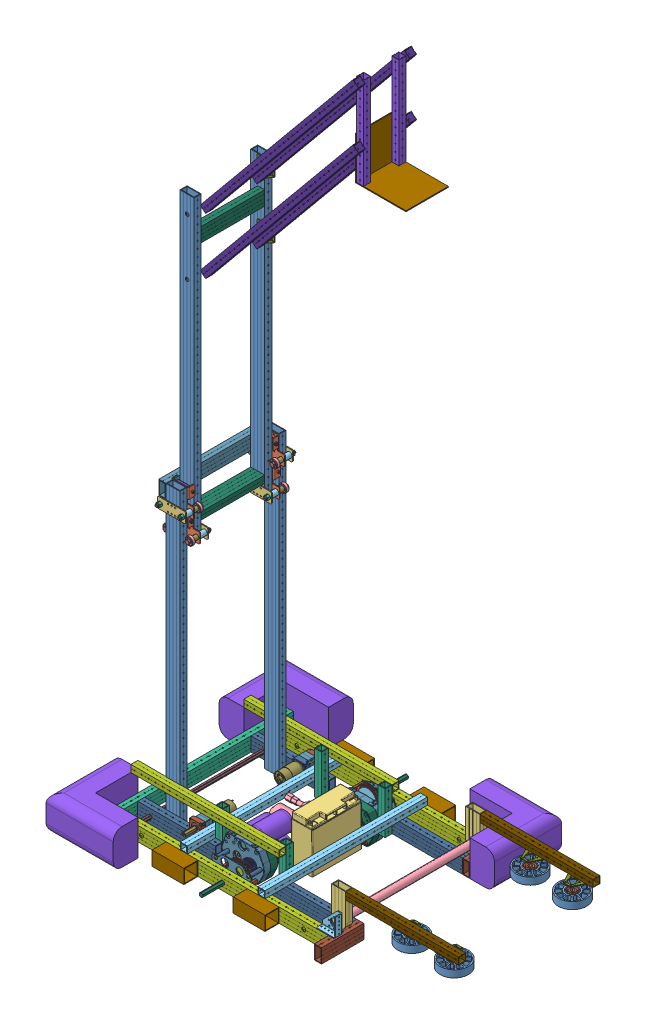
SolidWorks assembly Test Robot 2, configuration Default. Lengths in mm.
Overall size (1308.22 2664.65 863.6).
474 component instances, 122 part files, 52 mates.
Components (placement in the parent):
- Elevator Base Frame-1: Elevator Base Frame [Default] at (1458.6962 1126.0433 -272.9132) x (0 0 1) z (-1 0 0) size (419.1 1066.8 119.57)
  - Elevator Fixed Frame-1: Elevator Fixed Frame [Default] at (786.6435 8.8982 734.5957) x (1 0 0) z (0 1 0) size (25.4 50.8 1066.8)
  - Elevator Fixed Frame-2: Elevator Fixed Frame [Default] at (431.0435 8.8982 734.5957) x (1 0 0) z (0 1 0) size (25.4 50.8 1066.8)
  - am-3844+2x1+Elevator+Assembly+Example-1: am-3844+2x1+Elevator+Assembly+Example [Default] at (37.3435 1067.0077 761.7737) x (-1 0 0) z (0 0 1) size (82.37 89.82 113.91)
    - Example Single Corner Bearing Assembly-1: Example Single Corner Bearing Assembly [Default] at (-442.3285 289.2703 9.4128) x (0 0 1) z (-1 0 0) size (113.91 89.82 82.37)
      - Large Bearing Block Plate-1: Large Bearing Block Plate [Default] at (-85.6128 70.3392 -35.9285) x (1 0 0) z (0 -1 0) size (101.6 24.99 88.9)
      - Small Bearing Block Plate-1: Small Bearing Block Plate [Default] at (-85.6128 70.3392 -64.5035) x (1 0 0) z (0 -1 0) size (101.6 3.17 38.1)
      - 1614Z Bearing-1: 1614Z Bearing [Default] at (-74.6273 89.3892 -8.941) x (-0.590982 0.806685 0) z (0 0 1) size (28.58 28.58 9.53)
      - 1614Z Bearing-2: 1614Z Bearing [Default] at (5.0017 89.3892 -8.941) x (0.001674 0.999999 0) z (0 0 1) size (28.58 28.58 9.53)
      - AS75-18-64 Aluminum Spacer-1: AS75-18-64 Aluminum Spacer [Default] at (5.0017 89.3892 -35.9285) x (-0.668699 0.743533 0) z (-0.743533 -0.668699 0) size (19.05 25.41 19.05)
      - AS75-18-64 Aluminum Spacer-2: AS75-18-64 Aluminum Spacer [Default] at (-74.6273 89.3892 -61.3285) x (0.536222 0.844077 0) z (0.844077 -0.536222 0) size (19.05 25.41 19.05)
      - 3-8-16 NyLock Nut - Mcm 95615A140_95615A140-1: 3-8-16 NyLock Nut - Mcm 95615A140_95615A140 [Default] at (5.0017 89.3892 -64.5035) x (1 0 0) z (0 1 0) size (14.29 12 16.5)
      - 3-8-16 NyLock Nut - Mcm 95615A140_95615A140-2: 3-8-16 NyLock Nut - Mcm 95615A140_95615A140 [Default] at (-74.6273 89.3892 -64.5035) x (1 0 0) z (0 1 0) size (14.29 12 16.5)
      - am-0602 .250 x .192 x 2.14 Brass Tube-1: am-0602 .250 x .192 x 2.14 Brass Tube [Default] at (-7.6348 38.5892 -20.4599) x (0 0 1) z (-1 0 0) size (6.35 6.35 54.36)
      - 13RS075051 .750 x .260 x 1.00 Spacer-1: 13RS075051 .750 x .260 x 1.00 Spacer [Default] at (-60.2128 38.5892 -20.4599) x (0 -0.722855 0.691) z (0 0.691 0.722855) size (19.05 25.4 19.05)
      - 13RS075051 .750 x .260 x 1.00 Spacer-2: 13RS075051 .750 x .260 x 1.00 Spacer [Default] at (-34.8128 38.5892 -20.4599) x (0 -0.801304 -0.598258) z (0 -0.598258 0.801304) size (19.05 25.4 19.05)
      - 0.25 Flat Washer_Preferred Wide FW 0.25-1: 0.25 Flat Washer_Preferred Wide FW 0.25 [Default] at (-60.2128 38.5892 -20.4599) x (1 0 0) z (0 -0.116572 0.993182) size (1.4 15.88 15.88)
      - 0.25 Flat Washer_Preferred Wide FW 0.25-2: 0.25 Flat Washer_Preferred Wide FW 0.25 [Default] at (-8.0158 38.5892 -20.4599) size (1.4 15.88 15.88)
      - 10-32 Nylock Nut-1: 10-32 Nylock Nut [Default] at (-65.1658 38.5892 -20.4599) x (0 -0.097883 0.995198) z (-1 0 0) size (9.53 11 5.96)
      - SHCS 10-32 x 2.75_HX-SHCS 0.19-32x2.75x0.875-C-1: SHCS 10-32 x 2.75_HX-SHCS 0.19-32x2.75x0.875-C [Default] at (0.3662 38.5892 -20.4599) x (-1 0 0) z (0 0.982583 -0.185827) size (74.68 7.94 7.94)
      - AS62-18-56 Aluminum Spacer-1: AS62-18-56 Aluminum Spacer [Default] at (5.0017 89.3892 -13.7035) x (0.977193 0.212353 0) z (-0.212353 0.977193 0) size (15.88 19.06 15.88)
      - AS62-18-56 Aluminum Spacer-2: AS62-18-56 Aluminum Spacer [Default] at (-74.6273 89.3892 -13.7035) x (1 0 0) z (0 1 0) size (15.88 19.06 15.88)
      - 375-16 x 3 Hex Bolt_HFBOLT 0.375-16x2.5x1-C-1: 375-16 x 3 Hex Bolt_HFBOLT 0.375-16x2.5x1-C [Default] at (-74.6273 89.3892 1.9937) x (0 0 -1) z (1 0 0) size (82.37 16.48 14.28)
      - 375-16 x 3 Hex Bolt_HFBOLT 0.375-16x2.5x1-C-2: 375-16 x 3 Hex Bolt_HFBOLT 0.375-16x2.5x1-C [Default] at (5.0017 89.3892 1.9937) x (0 0 -1) z (-0.5 -0.866025 0) size (82.37 16.48 14.28)
  - am-3844+2x1+Elevator+Assembly+Example-2: am-3844+2x1+Elevator+Assembly+Example [Default] at (1180.3435 1067.0077 710.9737) x (1 0 0) z (0 0 -1) size (82.37 89.82 113.91)
    - Example Single Corner Bearing Assembly-1: Example Single Corner Bearing Assembly [Default] at (-442.3285 289.2703 9.4128) x (0 0 1) z (-1 0 0) size (113.91 89.82 82.37)
      - Large Bearing Block Plate-1: Large Bearing Block Plate [Default] at (-85.6128 70.3392 -35.9285) x (1 0 0) z (0 -1 0) size (101.6 24.99 88.9)
      - Small Bearing Block Plate-1: Small Bearing Block Plate [Default] at (-85.6128 70.3392 -64.5035) x (1 0 0) z (0 -1 0) size (101.6 3.17 38.1)
      - 1614Z Bearing-1: 1614Z Bearing [Default] at (-74.6273 89.3892 -8.941) x (-0.590982 0.806685 0) z (0 0 1) size (28.58 28.58 9.53)
      - 1614Z Bearing-2: 1614Z Bearing [Default] at (5.0017 89.3892 -8.941) x (0.001674 0.999999 0) z (0 0 1) size (28.58 28.58 9.53)
      - AS75-18-64 Aluminum Spacer-1: AS75-18-64 Aluminum Spacer [Default] at (5.0017 89.3892 -35.9285) x (-0.668699 0.743533 0) z (-0.743533 -0.668699 0) size (19.05 25.41 19.05)
      - AS75-18-64 Aluminum Spacer-2: AS75-18-64 Aluminum Spacer [Default] at (-74.6273 89.3892 -61.3285) x (0.536222 0.844077 0) z (0.844077 -0.536222 0) size (19.05 25.41 19.05)
      - 3-8-16 NyLock Nut - Mcm 95615A140_95615A140-1: 3-8-16 NyLock Nut - Mcm 95615A140_95615A140 [Default] at (5.0017 89.3892 -64.5035) x (1 0 0) z (0 1 0) size (14.29 12 16.5)
      - 3-8-16 NyLock Nut - Mcm 95615A140_95615A140-2: 3-8-16 NyLock Nut - Mcm 95615A140_95615A140 [Default] at (-74.6273 89.3892 -64.5035) x (1 0 0) z (0 1 0) size (14.29 12 16.5)
      - am-0602 .250 x .192 x 2.14 Brass Tube-1: am-0602 .250 x .192 x 2.14 Brass Tube [Default] at (-7.6348 38.5892 -20.4599) x (0 0 1) z (-1 0 0) size (6.35 6.35 54.36)
      - 13RS075051 .750 x .260 x 1.00 Spacer-1: 13RS075051 .750 x .260 x 1.00 Spacer [Default] at (-60.2128 38.5892 -20.4599) x (0 -0.722855 0.691) z (0 0.691 0.722855) size (19.05 25.4 19.05)
      - 13RS075051 .750 x .260 x 1.00 Spacer-2: 13RS075051 .750 x .260 x 1.00 Spacer [Default] at (-34.8128 38.5892 -20.4599) x (0 -0.801304 -0.598258) z (0 -0.598258 0.801304) size (19.05 25.4 19.05)
      - 0.25 Flat Washer_Preferred Wide FW 0.25-1: 0.25 Flat Washer_Preferred Wide FW 0.25 [Default] at (-60.2128 38.5892 -20.4599) x (1 0 0) z (0 -0.116572 0.993182) size (1.4 15.88 15.88)
      - 0.25 Flat Washer_Preferred Wide FW 0.25-2: 0.25 Flat Washer_Preferred Wide FW 0.25 [Default] at (-8.0158 38.5892 -20.4599) size (1.4 15.88 15.88)
      - 10-32 Nylock Nut-1: 10-32 Nylock Nut [Default] at (-65.1658 38.5892 -20.4599) x (0 -0.097883 0.995198) z (-1 0 0) size (9.53 11 5.96)
      - SHCS 10-32 x 2.75_HX-SHCS 0.19-32x2.75x0.875-C-1: SHCS 10-32 x 2.75_HX-SHCS 0.19-32x2.75x0.875-C [Default] at (0.3662 38.5892 -20.4599) x (-1 0 0) z (0 0.982583 -0.185827) size (74.68 7.94 7.94)
      - AS62-18-56 Aluminum Spacer-1: AS62-18-56 Aluminum Spacer [Default] at (5.0017 89.3892 -13.7035) x (0.977193 0.212353 0) z (-0.212353 0.977193 0) size (15.88 19.06 15.88)
      - AS62-18-56 Aluminum Spacer-2: AS62-18-56 Aluminum Spacer [Default] at (-74.6273 89.3892 -13.7035) x (1 0 0) z (0 1 0) size (15.88 19.06 15.88)
      - 375-16 x 3 Hex Bolt_HFBOLT 0.375-16x2.5x1-C-1: 375-16 x 3 Hex Bolt_HFBOLT 0.375-16x2.5x1-C [Default] at (-74.6273 89.3892 1.9937) x (0 0 -1) z (1 0 0) size (82.37 16.48 14.28)
      - 375-16 x 3 Hex Bolt_HFBOLT 0.375-16x2.5x1-C-2: 375-16 x 3 Hex Bolt_HFBOLT 0.375-16x2.5x1-C [Default] at (5.0017 89.3892 1.9937) x (0 0 -1) z (-0.5 -0.866025 0) size (82.37 16.48 14.28)
  - Frame Crossbar-1: Frame Crossbar [Default] at (1167.6435 732.7982 772.6957) x (0 0 1) z (-1 0 0) size (25.4 50.8 381)
- Elevator Moving Stage-1: Elevator Moving Stage [Default] at (-203.0913 2022.1821 901.5512) x (0 0 -1) z (1 0 0) size (355.24 1067.72 119.92)
  - Elevator Fixed Frame-1: Elevator Fixed Frame [Default] at (692.621 1.7594 927.1918) x (1 0 0) z (0 1 0) size (25.4 50.8 1066.8)
  - Elevator Fixed Frame-2: Elevator Fixed Frame [Default] at (438.621 1.7594 927.1918) x (1 0 0) z (0 1 0) size (25.4 50.8 1066.8)
  - Elevator Crossbar-1: Elevator Crossbar [Default] at (1200.621 -252.2406 927.1918) x (0 -1 0) z (-1 0 0) size (25.4 50.8 228.6)
  - am-3844+2x1+Elevator+Assembly+Example-1: am-3844+2x1+Elevator+Assembly+Example [Default] at (298.921 81.9689 954.3698) x (-1 0 0) z (0 0 1) size (82.37 89.82 113.91)
    - Example Single Corner Bearing Assembly-1: Example Single Corner Bearing Assembly [Default] at (-442.3285 289.2703 9.4128) x (0 0 1) z (-1 0 0) size (113.91 89.82 82.37)
      - Large Bearing Block Plate-1: Large Bearing Block Plate [Default] at (-85.6128 70.3392 -35.9285) x (1 0 0) z (0 -1 0) size (101.6 24.99 88.9)
      - Small Bearing Block Plate-1: Small Bearing Block Plate [Default] at (-85.6128 70.3392 -64.5035) x (1 0 0) z (0 -1 0) size (101.6 3.17 38.1)
      - 1614Z Bearing-1: 1614Z Bearing [Default] at (-74.6273 89.3892 -8.941) x (-0.590982 0.806685 0) z (0 0 1) size (28.58 28.58 9.53)
      - 1614Z Bearing-2: 1614Z Bearing [Default] at (5.0017 89.3892 -8.941) x (0.001674 0.999999 0) z (0 0 1) size (28.58 28.58 9.53)
      - AS75-18-64 Aluminum Spacer-1: AS75-18-64 Aluminum Spacer [Default] at (5.0017 89.3892 -35.9285) x (-0.668699 0.743533 0) z (-0.743533 -0.668699 0) size (19.05 25.41 19.05)
      - AS75-18-64 Aluminum Spacer-2: AS75-18-64 Aluminum Spacer [Default] at (-74.6273 89.3892 -61.3285) x (0.536222 0.844077 0) z (0.844077 -0.536222 0) size (19.05 25.41 19.05)
      - 3-8-16 NyLock Nut - Mcm 95615A140_95615A140-1: 3-8-16 NyLock Nut - Mcm 95615A140_95615A140 [Default] at (5.0017 89.3892 -64.5035) x (1 0 0) z (0 1 0) size (14.29 12 16.5)
      - 3-8-16 NyLock Nut - Mcm 95615A140_95615A140-2: 3-8-16 NyLock Nut - Mcm 95615A140_95615A140 [Default] at (-74.6273 89.3892 -64.5035) x (1 0 0) z (0 1 0) size (14.29 12 16.5)
      - am-0602 .250 x .192 x 2.14 Brass Tube-1: am-0602 .250 x .192 x 2.14 Brass Tube [Default] at (-7.6348 38.5892 -20.4599) x (0 0 1) z (-1 0 0) size (6.35 6.35 54.36)
      - 13RS075051 .750 x .260 x 1.00 Spacer-1: 13RS075051 .750 x .260 x 1.00 Spacer [Default] at (-60.2128 38.5892 -20.4599) x (0 -0.722855 0.691) z (0 0.691 0.722855) size (19.05 25.4 19.05)
      - 13RS075051 .750 x .260 x 1.00 Spacer-2: 13RS075051 .750 x .260 x 1.00 Spacer [Default] at (-34.8128 38.5892 -20.4599) x (0 -0.801304 -0.598258) z (0 -0.598258 0.801304) size (19.05 25.4 19.05)
      - 0.25 Flat Washer_Preferred Wide FW 0.25-1: 0.25 Flat Washer_Preferred Wide FW 0.25 [Default] at (-60.2128 38.5892 -20.4599) x (1 0 0) z (0 -0.116572 0.993182) size (1.4 15.88 15.88)
      - 0.25 Flat Washer_Preferred Wide FW 0.25-2: 0.25 Flat Washer_Preferred Wide FW 0.25 [Default] at (-8.0158 38.5892 -20.4599) size (1.4 15.88 15.88)
      - 10-32 Nylock Nut-1: 10-32 Nylock Nut [Default] at (-65.1658 38.5892 -20.4599) x (0 -0.097883 0.995198) z (-1 0 0) size (9.53 11 5.96)
      - SHCS 10-32 x 2.75_HX-SHCS 0.19-32x2.75x0.875-C-1: SHCS 10-32 x 2.75_HX-SHCS 0.19-32x2.75x0.875-C [Default] at (0.3662 38.5892 -20.4599) x (-1 0 0) z (0 0.982583 -0.185827) size (74.68 7.94 7.94)
      - AS62-18-56 Aluminum Spacer-1: AS62-18-56 Aluminum Spacer [Default] at (5.0017 89.3892 -13.7035) x (0.977193 0.212353 0) z (-0.212353 0.977193 0) size (15.88 19.06 15.88)
      - AS62-18-56 Aluminum Spacer-2: AS62-18-56 Aluminum Spacer [Default] at (-74.6273 89.3892 -13.7035) x (1 0 0) z (0 1 0) size (15.88 19.06 15.88)
      - 375-16 x 3 Hex Bolt_HFBOLT 0.375-16x2.5x1-C-1: 375-16 x 3 Hex Bolt_HFBOLT 0.375-16x2.5x1-C [Default] at (-74.6273 89.3892 1.9937) x (0 0 -1) z (1 0 0) size (82.37 16.48 14.28)
      - 375-16 x 3 Hex Bolt_HFBOLT 0.375-16x2.5x1-C-2: 375-16 x 3 Hex Bolt_HFBOLT 0.375-16x2.5x1-C [Default] at (5.0017 89.3892 1.9937) x (0 0 -1) z (-0.5 -0.866025 0) size (82.37 16.48 14.28)
  - am-3844+2x1+Elevator+Assembly+Example-2: am-3844+2x1+Elevator+Assembly+Example [Default] at (832.321 81.9689 900.0138) x (1 0 0) z (0 0 -1) size (82.37 89.82 113.91)
    - Example Single Corner Bearing Assembly-1: Example Single Corner Bearing Assembly [Default] at (-442.3285 289.2703 9.4128) x (0 0 1) z (-1 0 0) size (113.91 89.82 82.37)
      - Large Bearing Block Plate-1: Large Bearing Block Plate [Default] at (-85.6128 70.3392 -35.9285) x (1 0 0) z (0 -1 0) size (101.6 24.99 88.9)
      - Small Bearing Block Plate-1: Small Bearing Block Plate [Default] at (-85.6128 70.3392 -64.5035) x (1 0 0) z (0 -1 0) size (101.6 3.17 38.1)
      - 1614Z Bearing-1: 1614Z Bearing [Default] at (-74.6273 89.3892 -8.941) x (-0.590982 0.806685 0) z (0 0 1) size (28.58 28.58 9.53)
      - 1614Z Bearing-2: 1614Z Bearing [Default] at (5.0017 89.3892 -8.941) x (0.001674 0.999999 0) z (0 0 1) size (28.58 28.58 9.53)
      - AS75-18-64 Aluminum Spacer-1: AS75-18-64 Aluminum Spacer [Default] at (5.0017 89.3892 -35.9285) x (-0.668699 0.743533 0) z (-0.743533 -0.668699 0) size (19.05 25.41 19.05)
      - AS75-18-64 Aluminum Spacer-2: AS75-18-64 Aluminum Spacer [Default] at (-74.6273 89.3892 -61.3285) x (0.536222 0.844077 0) z (0.844077 -0.536222 0) size (19.05 25.41 19.05)
      - 3-8-16 NyLock Nut - Mcm 95615A140_95615A140-1: 3-8-16 NyLock Nut - Mcm 95615A140_95615A140 [Default] at (5.0017 89.3892 -64.5035) x (1 0 0) z (0 1 0) size (14.29 12 16.5)
      - 3-8-16 NyLock Nut - Mcm 95615A140_95615A140-2: 3-8-16 NyLock Nut - Mcm 95615A140_95615A140 [Default] at (-74.6273 89.3892 -64.5035) x (1 0 0) z (0 1 0) size (14.29 12 16.5)
      - am-0602 .250 x .192 x 2.14 Brass Tube-1: am-0602 .250 x .192 x 2.14 Brass Tube [Default] at (-7.6348 38.5892 -20.4599) x (0 0 1) z (-1 0 0) size (6.35 6.35 54.36)
      - 13RS075051 .750 x .260 x 1.00 Spacer-1: 13RS075051 .750 x .260 x 1.00 Spacer [Default] at (-60.2128 38.5892 -20.4599) x (0 -0.722855 0.691) z (0 0.691 0.722855) size (19.05 25.4 19.05)
      - 13RS075051 .750 x .260 x 1.00 Spacer-2: 13RS075051 .750 x .260 x 1.00 Spacer [Default] at (-34.8128 38.5892 -20.4599) x (0 -0.801304 -0.598258) z (0 -0.598258 0.801304) size (19.05 25.4 19.05)
      - 0.25 Flat Washer_Preferred Wide FW 0.25-1: 0.25 Flat Washer_Preferred Wide FW 0.25 [Default] at (-60.2128 38.5892 -20.4599) x (1 0 0) z (0 -0.116572 0.993182) size (1.4 15.88 15.88)
      - 0.25 Flat Washer_Preferred Wide FW 0.25-2: 0.25 Flat Washer_Preferred Wide FW 0.25 [Default] at (-8.0158 38.5892 -20.4599) size (1.4 15.88 15.88)
      - 10-32 Nylock Nut-1: 10-32 Nylock Nut [Default] at (-65.1658 38.5892 -20.4599) x (0 -0.097883 0.995198) z (-1 0 0) size (9.53 11 5.96)
      - SHCS 10-32 x 2.75_HX-SHCS 0.19-32x2.75x0.875-C-1: SHCS 10-32 x 2.75_HX-SHCS 0.19-32x2.75x0.875-C [Default] at (0.3662 38.5892 -20.4599) x (-1 0 0) z (0 0.982583 -0.185827) size (74.68 7.94 7.94)
      - AS62-18-56 Aluminum Spacer-1: AS62-18-56 Aluminum Spacer [Default] at (5.0017 89.3892 -13.7035) x (0.977193 0.212353 0) z (-0.212353 0.977193 0) size (15.88 19.06 15.88)
      - AS62-18-56 Aluminum Spacer-2: AS62-18-56 Aluminum Spacer [Default] at (-74.6273 89.3892 -13.7035) x (1 0 0) z (0 1 0) size (15.88 19.06 15.88)
      - 375-16 x 3 Hex Bolt_HFBOLT 0.375-16x2.5x1-C-1: 375-16 x 3 Hex Bolt_HFBOLT 0.375-16x2.5x1-C [Default] at (-74.6273 89.3892 1.9937) x (0 0 -1) z (1 0 0) size (82.37 16.48 14.28)
      - 375-16 x 3 Hex Bolt_HFBOLT 0.375-16x2.5x1-C-2: 375-16 x 3 Hex Bolt_HFBOLT 0.375-16x2.5x1-C [Default] at (5.0017 89.3892 1.9937) x (0 0 -1) z (-0.5 -0.866025 0) size (82.37 16.48 14.28)
  - VersaFrame Side Bearing Mount-1: VersaFrame Side Bearing Mount [Default] at (677.635 719.3094 968.4668) x (0 -1 0) z (1 0 0) size (63.5 61.91 2.29)
  - Elevator Crossbar-2: Elevator Crossbar [Default] at (-69.379 624.0594 939.8918) x (0 0 -1) z (1 0 0) size (25.4 50.8 228.6)
  - VersaFrame Side Bearing Mount-2: VersaFrame Side Bearing Mount [Default] at (677.635 516.1094 968.4668) x (0 -1 0) z (1 0 0) size (63.5 61.91 2.29)
- Elevator Arm Section-1: Elevator Arm Section [Default] at (1226.325 3096.4643 431.1803) x (-0.771063 0.636758 0) z (-0.636758 -0.771063 0) size (25.4 25.4 863.6)
- Elevator Arm Section-2: Elevator Arm Section [Default] at (1226.325 3299.6643 431.1803) x (-0.771063 0.636758 0) z (-0.636758 -0.771063 0) size (25.4 25.4 863.6)
- Elevator Arm Section-3: Elevator Arm Section [Default] at (1226.325 3299.6643 247.0303) x (-0.771063 0.636758 0) z (-0.636758 -0.771063 0) size (25.4 25.4 863.6)
- Elevator Arm Section-4: Elevator Arm Section [Default] at (1226.325 3096.4643 247.0303) x (-0.771063 0.636758 0) z (-0.636758 -0.771063 0) size (25.4 25.4 863.6)
- Intake Mechanism-2: Intake Mechanism [Default] at (762.7163 825.0983 733.2058) x (-1 0 0) z (0 0 -1) size (127 459.2 565.18) (hidden)
  - Intake Arm-1: Intake Arm [Default] at (166.6282 -436.1132 702.0756) x (0 0 1) z (0 1 0) size (25.4 25.4 406.4)
  - am-3480+4IN+500Hex+Bore+Compliant+Wheel-1: am-3480+4IN+500Hex+Bore+Compliant+Wheel [Default] at (107.5902 -52.3006 677.3515) x (0 -1 0) z (1 0 0) size (101.6 101.6 25.74)
    - 4IN Compliant Wheel FINAL Overmold-1: 4IN Compliant Wheel FINAL Overmold [Default] at (-16.2374 3.8509 18.652) size (101.6 101.6 25.74)
    - 2in Wheel Intergrated 0500 HEX Hub-1: 2in Wheel Intergrated 0500 HEX Hub [Default] at (-16.2374 3.8509 5.952) x (-1 0 0) z (0 0 -1) size (41.91 41.91 25.4)
  - VersaFrame Side Bearing Mount-1: VersaFrame Side Bearing Mount [Default] at (151.6422 -36.0632 673.5006) x (0 1 0) z (1 0 0) size (63.5 61.91 2.29)
  - am-3480+4IN+500Hex+Bore+Compliant+Wheel-2: am-3480+4IN+500Hex+Bore+Compliant+Wheel [Default] at (107.5902 102.0213 664.9245) x (0 -0.716102 -0.697996) z (1 0 0) size (101.6 101.6 25.74)
    - 4IN Compliant Wheel FINAL Overmold-1: 4IN Compliant Wheel FINAL Overmold [Default] at (-16.2374 3.8509 18.652) size (101.6 101.6 25.74)
    - 2in Wheel Intergrated 0500 HEX Hub-1: 2in Wheel Intergrated 0500 HEX Hub [Default] at (-16.2374 3.8509 5.952) x (-1 0 0) z (0 0 -1) size (41.91 41.91 25.4)
  - VersaFrame Side Bearing Mount-2: VersaFrame Side Bearing Mount [Default] at (151.6422 116.3368 673.5006) x (0 1 0) z (1 0 0) size (63.5 61.91 2.29)
  - VersaFrame Side Bearing Mount-3: VersaFrame Side Bearing Mount [Default] at (151.6422 -36.0632 248.0506) x (0 -1 0) z (1 0 0) size (63.5 61.91 2.29)
  - am-3480+4IN+500Hex+Bore+Compliant+Wheel-3: am-3480+4IN+500Hex+Bore+Compliant+Wheel [Default] at (107.5902 103.4135 258.6086) x (0 -0.899512 0.436896) z (1 0 0) size (101.6 101.6 25.74)
    - 4IN Compliant Wheel FINAL Overmold-1: 4IN Compliant Wheel FINAL Overmold [Default] at (-16.2374 3.8509 18.652) size (101.6 101.6 25.74)
    - 2in Wheel Intergrated 0500 HEX Hub-1: 2in Wheel Intergrated 0500 HEX Hub [Default] at (-16.2374 3.8509 5.952) x (-1 0 0) z (0 0 -1) size (41.91 41.91 25.4)
  - VersaFrame Side Bearing Mount-4: VersaFrame Side Bearing Mount [Default] at (151.6422 116.3368 248.0506) x (0 -1 0) z (1 0 0) size (63.5 61.91 2.29)
  - am-3480+4IN+500Hex+Bore+Compliant+Wheel-4: am-3480+4IN+500Hex+Bore+Compliant+Wheel [Default] at (107.5902 -19.397 247.2002) x (0 0.983506 0.180877) z (1 0 0) size (101.6 101.6 25.74)
    - 4IN Compliant Wheel FINAL Overmold-1: 4IN Compliant Wheel FINAL Overmold [Default] at (-16.2374 3.8509 18.652) size (101.6 101.6 25.74)
    - 2in Wheel Intergrated 0500 HEX Hub-1: 2in Wheel Intergrated 0500 HEX Hub [Default] at (-16.2374 3.8509 5.952) x (-1 0 0) z (0 0 -1) size (41.91 41.91 25.4)
  - Intake Arm-2: Intake Arm [Default] at (166.6282 -436.1132 219.4756) x (0 0 1) z (0 1 0) size (25.4 25.4 406.4)
  - Intake Upright 2-1: Intake Upright 2 [Default] at (801.6282 338.5868 219.4756) x (0 0 1) z (-1 0 0) size (25.4 50.8 127)
  - Intake Upright 2-2: Intake Upright 2 [Default] at (801.6282 338.5868 702.0756) x (0 0 1) z (-1 0 0) size (25.4 50.8 127)
  - Intake Round Crossbar-1: Intake Round Crossbar [Default] at (77.7282 338.663 232.1756) size (25.4 25.4 457.2)
- Intake Mechanism-3: Intake Mechanism [Default] at (1721.2035 817.8734 -125.8193) x (0 1 0) z (0 0 1) size (127 459.2 565.18)
  - Intake Arm-1: Intake Arm [Default] at (166.6282 -436.1132 702.0756) x (0 0 1) z (0 1 0) size (25.4 25.4 406.4)
  - am-3480+4IN+500Hex+Bore+Compliant+Wheel-1: am-3480+4IN+500Hex+Bore+Compliant+Wheel [Default] at (107.5902 -52.3006 677.3515) x (0 -1 0) z (1 0 0) size (101.6 101.6 25.74)
    - 4IN Compliant Wheel FINAL Overmold-1: 4IN Compliant Wheel FINAL Overmold [Default] at (-16.2374 3.8509 18.652) size (101.6 101.6 25.74)
    - 2in Wheel Intergrated 0500 HEX Hub-1: 2in Wheel Intergrated 0500 HEX Hub [Default] at (-16.2374 3.8509 5.952) x (-1 0 0) z (0 0 -1) size (41.91 41.91 25.4)
  - VersaFrame Side Bearing Mount-1: VersaFrame Side Bearing Mount [Default] at (151.6422 -36.0632 673.5006) x (0 1 0) z (1 0 0) size (63.5 61.91 2.29)
  - am-3480+4IN+500Hex+Bore+Compliant+Wheel-2: am-3480+4IN+500Hex+Bore+Compliant+Wheel [Default] at (107.5902 102.0213 664.9245) x (0 -0.716102 -0.697996) z (1 0 0) size (101.6 101.6 25.74)
    - 4IN Compliant Wheel FINAL Overmold-1: 4IN Compliant Wheel FINAL Overmold [Default] at (-16.2374 3.8509 18.652) size (101.6 101.6 25.74)
    - 2in Wheel Intergrated 0500 HEX Hub-1: 2in Wheel Intergrated 0500 HEX Hub [Default] at (-16.2374 3.8509 5.952) x (-1 0 0) z (0 0 -1) size (41.91 41.91 25.4)
  - VersaFrame Side Bearing Mount-2: VersaFrame Side Bearing Mount [Default] at (151.6422 116.3368 673.5006) x (0 1 0) z (1 0 0) size (63.5 61.91 2.29)
  - VersaFrame Side Bearing Mount-3: VersaFrame Side Bearing Mount [Default] at (151.6422 -36.0632 248.0506) x (0 -1 0) z (1 0 0) size (63.5 61.91 2.29)
  - am-3480+4IN+500Hex+Bore+Compliant+Wheel-3: am-3480+4IN+500Hex+Bore+Compliant+Wheel [Default] at (107.5902 103.4135 258.6086) x (0 -0.899512 0.436896) z (1 0 0) size (101.6 101.6 25.74)
    - 4IN Compliant Wheel FINAL Overmold-1: 4IN Compliant Wheel FINAL Overmold [Default] at (-16.2374 3.8509 18.652) size (101.6 101.6 25.74)
    - 2in Wheel Intergrated 0500 HEX Hub-1: 2in Wheel Intergrated 0500 HEX Hub [Default] at (-16.2374 3.8509 5.952) x (-1 0 0) z (0 0 -1) size (41.91 41.91 25.4)
  - VersaFrame Side Bearing Mount-4: VersaFrame Side Bearing Mount [Default] at (151.6422 116.3368 248.0506) x (0 -1 0) z (1 0 0) size (63.5 61.91 2.29)
  - am-3480+4IN+500Hex+Bore+Compliant+Wheel-4: am-3480+4IN+500Hex+Bore+Compliant+Wheel [Default] at (107.5902 -19.397 247.2002) x (0 0.983506 0.180877) z (1 0 0) size (101.6 101.6 25.74)
    - 4IN Compliant Wheel FINAL Overmold-1: 4IN Compliant Wheel FINAL Overmold [Default] at (-16.2374 3.8509 18.652) size (101.6 101.6 25.74)
    - 2in Wheel Intergrated 0500 HEX Hub-1: 2in Wheel Intergrated 0500 HEX Hub [Default] at (-16.2374 3.8509 5.952) x (-1 0 0) z (0 0 -1) size (41.91 41.91 25.4)
  - Intake Arm-2: Intake Arm [Default] at (166.6282 -436.1132 219.4756) x (0 0 1) z (0 1 0) size (25.4 25.4 406.4)
  - Intake Upright 2-1: Intake Upright 2 [Default] at (801.6282 338.5868 219.4756) x (0 0 1) z (-1 0 0) size (25.4 50.8 127)
  - Intake Upright 2-2: Intake Upright 2 [Default] at (801.6282 338.5868 702.0756) x (0 0 1) z (-1 0 0) size (25.4 50.8 127)
  - Intake Round Crossbar-1: Intake Round Crossbar [Default] at (77.7282 338.663 232.1756) size (25.4 25.4 457.2)
- VersaFrame Corner Gusset-1: VersaFrame Corner Gusset [Default] at (1409.9006 868.2415 68.2563) x (-1 0 0) z (0 0 -1) size (69.72 69.72 25.4)
- Test Base 2-1: Test Base 2 [Default] at (327.6786 481.923 -175.606) size (990.6 253.34 863.6)
  - Base Rear Rail-1: Base Rear Rail [Default] at (282.1219 360.9185 104.1623) size (25.4 50.8 685.8)
  - Base Side Rail-1: Base Side Rail [Default] at (1044.1219 360.9185 789.9623) x (0 0 1) z (-1 0 0) size (25.4 50.8 762)
  - Base Side Rail-2: Base Side Rail [Default] at (1044.1219 360.9185 231.1623) x (0 0 1) z (-1 0 0) size (25.4 50.8 762)
  - Blue Bumper-1: Blue Bumper [Default] at (1171.1219 335.5185 942.3623) x (0 0 -1) z (1 0 0) size (241.3 127 241.3) (hidden)
  - Blue Bumper-2: Blue Bumper [Default] at (1171.1219 335.5185 78.7623) x (-1 0 0) z (0 0 -1) size (241.3 127 241.3)
  - Bumper Support Bar-2: Bumper Support Bar [Default] at (879.0219 335.5185 166.0294) x (0 0 1) z (-1 0 0) size (50.8 50.8 114.3)
  - Bumper Support Bar-4: Bumper Support Bar [Default] at (586.9219 335.5185 166.0294) x (0 0 1) z (-1 0 0) size (50.8 50.8 114.3)
  - Bumper Support Bar-7: Bumper Support Bar [Default] at (586.9219 335.5185 801.0294) x (0 0 1) z (-1 0 0) size (50.8 50.8 114.3)
  - Bumper Support Bar-8: Bumper Support Bar [Default] at (879.0219 335.5185 801.0294) x (0 0 1) z (-1 0 0) size (50.8 50.8 114.3)
  - Base Side Rail Internal-1: Base Side Rail Internal [Default] at (-175.0781 360.9185 307.3623) x (0 0 -1) z (1 0 0) size (25.4 50.8 279.4)
  - Base Side Rail Internal-4: Base Side Rail Internal [Default] at (1044.1219 360.9185 714.7363) x (0 0 1) z (-1 0 0) size (25.4 50.8 279.4)
  - Base Front Rail-1: Base Front Rail [Default] at (1069.5219 360.9185 104.1623) size (25.4 50.8 152.4)
  - 3 CIM Ball Shifter with WCD Output-1: 3 CIM Ball Shifter with WCD Output [Default] at (711.3612 400.7203 682.3171) x (0 1 0) z (0 0 1) size (169.11 183.68 312.65)
    - 217-2733-001 Rev2-1: 217-2733-001 Rev2 [Default] at (0 53.4162 37.6682) x (0 0 1) z (-0.00054 -1 0) size (7.11 24.61 24.61)
    - 217-2733-001 Rev2-2: 217-2733-001 Rev2 [Default] at (0 53.4162 7.9248) x (0 0 -1) z (-0.038475 0.99926 0) size (7.11 24.61 24.61)
    - 217-2731-001 Rev2-1: 217-2731-001 Rev2 [Default] at (0 0 0.0381) x (-0.099212 0.995066 0) z (0.995066 0.099212 0) size (31.12 7.94 31.12)
    - 217-2789-001 Rev2-1: 217-2789-001 Rev2 [Default] at (0 0 43.2943) x (0 0 -1) z (-0.58471 0.811243 0) size (11.1 38.4 38.4)
    - 217-2778-001 Rev2_NCQ8A075-050M_1-1: 217-2778-001 Rev2_NCQ8A075-050M_1 [Default] at (0 0 -53.848) x (-0.707107 0.707107 0) z (0 0 1) size (31.75 33.34 39.88)
      - 217-2778-002_075A-1: 217-2778-002_075A [Default] at origin size (31.75 33.34 26.92)
      - 217-2778-003_075M-1: 217-2778-003_075M [Default] at (0 0 -8.85) x (0.866025 -0.5 0) z (0 0 1) size (18.95 18.95 35.27)
      - 217-2778-004_075-1: 217-2778-004_075 [Default] at (0 0 10.362) size (21 20.74 0.97)
    - 217-2428-012 Rev2-1: 217-2428-012 Rev2 [Default] at (0 0 -40.386) size (63.5 22.23 2.29)
    - 217-2428-005 Rev1-1: 217-2428-005 Rev1 [Default] at (25.4 0 -19.05) x (-0.557362 -0.83027 0) z (-0.83027 0.557362 0) size (7.33 38.98 6.35)
    - 217-2428-005 Rev1-2: 217-2428-005 Rev1 [Default] at (-25.4 0 -19.05) x (0.667436 0.744667 0) z (0.744667 -0.667436 0) size (7.33 38.98 6.35)
    - SCREW-832-0375-1: SCREW-832-0375 [Default] at (25.4 0 -42.5958) x (0 0 1) z (-0.875404 0.483392 0) size (11.73 7.92 7.92)
    - SCREW-832-0375-2: SCREW-832-0375 [Default] at (-25.4 0 -42.5958) x (0 0 1) z (-0.966319 0.257347 0) size (11.73 7.92 7.92)
    - SCREW-832-0375-3: SCREW-832-0375 [Default] at (25.4 0 5.3848) x (0 0 -1) z (1 0 0) size (11.73 7.92 7.92)
    - SCREW-832-0375-4: SCREW-832-0375 [Default] at (-25.4 0 5.3848) x (0 0 -1) z (0.941463 -0.337115 0) size (11.73 7.92 7.92)
    - SBS1_SBS-0632-0250-1: SBS1_SBS-0632-0250 [Default] at (15.494 0 -36.2458) x (0 0 -1) z (0.854303 -0.519775 0) size (8.57 6.68 6.65)
    - SBS1_SBS-0632-0250-2: SBS1_SBS-0632-0250 [Default] at (-15.494 0 -36.2458) x (0 0 -1) z (0.854303 -0.519775 0) size (8.57 6.68 6.65)
    - 217-4098-100 Rev1-1: 217-4098-100 Rev1 [Default] at (0 0 -16.927) x (-0.503316 0.864103 0) z (0 0 1) size (18.03 19.79 22.46)
      - 217-4098-006 Rev2-1: 217-4098-006 Rev2 [Default] at (0 0 -4.6312) x (0 -1 0) z (0 0 -1) size (18.09 11.02 22.46)
      - 217-4098-006 Rev2-2: 217-4098-006 Rev2 [Default] at (0 0 -4.6312) x (0 1 0) z (0 0 -1) size (18.09 11.02 22.46)
      - 217-3489-001 Rev1-1: 217-3489-001 Rev1 [Default] at (0 0 -4.6312) x (0 0 1) z (-0.980217 -0.197926 0) size (4.77 12.7 12.7)
      - 97633A130_97633A130_grv-1: 97633A130_97633A130_grv [Default] at (0 0 -7.33) x (0 0 -1) z (0.979861 0.199683 0) size (0.64 8.74 7.34)
      - 91251A107_91251A107-1: 91251A107_91251A107 [Default] at (-4.8375 -6.735 -9.4343) x (0 0.863883 -0.503692) z (-1 0 0) size (4.65 4.65 10.79)
      - 91251A107_91251A107-2: 91251A107_91251A107 [Default] at (4.8375 6.735 -9.4343) x (0 0.470889 -0.882193) z (1 0 0) size (4.65 4.65 10.79)
    - 217-2428-017 Rev2-1: 217-2428-017 Rev2 [Default] at (12.7 -21.997 -3.614) x (-0.578458 -0.815712 0) z (0 0 -1) size (14.73 14.73 7.37)
    - 217-2428-016 Rev3_Spur01-1: 217-2428-016 Rev3_Spur01 [Default] at (0 0 -3.614) x (0.873157 -0.48744 0) z (0 0 1) size (40.67 40.74 13.32)
    - 217-2428-019 Rev1-1: 217-2428-019 Rev1 [Default] at (12.7 -21.997 -20.6248) x (0.866025 0.5 0) z (0 0 1) size (50.8 19.05 1.57)
    - 217-2428-006 Rev1-1: 217-2428-006 Rev1 [Default] at (32.079 -14.2875 -9.525) x (-0.752416 0.658689 0) z (0.658689 0.752416 0) size (7.33 19.93 6.35)
    - 217-2428-006 Rev1-2: 217-2428-006 Rev1 [Default] at (-3.6662 -34.925 -9.525) x (0.84498 0.534798 0) z (0.534798 -0.84498 0) size (7.33 19.93 6.35)
    - SCREW-832-0375-5: SCREW-832-0375 [Default] at (32.079 -14.2875 4.7498) x (0 0 -1) z (0.980613 0.195955 0) size (11.73 7.92 7.92)
    - SCREW-832-0375-6: SCREW-832-0375 [Default] at (-3.6662 -34.925 5.3848) x (0 0 -1) z (-0.672515 -0.740083 0) size (11.73 7.92 7.92)
    - SCREW-832-0375-7: SCREW-832-0375 [Default] at (-3.6662 -34.925 -22.8346) x (0 0 1) z (0.948865 0.315681 0) size (11.73 7.92 7.92)
    - SCREW-832-0375-8: SCREW-832-0375 [Default] at (32.079 -14.2875 -22.8346) x (0 0 1) z (-0.875404 0.483392 0) size (11.73 7.92 7.92)
    - 217-2614-001_12t-1: 217-2614-001_12t [Default] at (36.9798 39.6868 15.8623) x (-0.087156 0.996195 0) z (0 0 1) size (18.29 18.29 19)
    - 217-2761-001 rev1-1: 217-2761-001 rev1 [Default] at (33.1943 39.3556 16.1) x (0.087156 -0.996195 0) z (0 0 1) size (2 2 20)
    - 217-2761-001 rev1-2: 217-2761-001 rev1 [Default] at (-40.7653 40.018 16.1) x (0.087156 0.996195 0) z (0 0 1) size (2 2 20)
    - 217-2614-001_12t-2: 217-2614-001_12t [Default] at (-36.9798 39.6868 15.8623) x (0.087156 0.996195 0) z (0 0 1) size (18.29 18.29 19)
    - 217-2614-001_12t-3: 217-2614-001_12t [Default] at (0 92.8624 15.8623) x (0.97459 0.223996 0) z (0 0 1) size (18.29 18.29 19)
    - 217-2761-001 rev1-3: 217-2761-001 rev1 [Default] at (-0.8512 96.5658 16.1) x (0.97459 0.223996 0) z (0 0 1) size (2 2 20)
    - 217-3195-002 rev2-1: 217-3195-002 rev2 [Default] at (0 0 50.546) x (-1 0 0) z (0 0 -1) size (114.31 152.24 24.96)
    - 217-3195-001 Rev1-1: 217-3195-001 Rev1 [Default] at origin size (113.41 152.24 26.86)
    - Nylock Nut_NNY2520-ZC-1: Nylock Nut_NNY2520-ZC [Default] at (48.8823 73.025 37.846) x (0 0.866025 -0.5) z (-1 0 0) size (12.85 11.89 7.62)
    - Nylock Nut_NNY2520-ZC-2: Nylock Nut_NNY2520-ZC [Default] at (48.8823 -3.175 37.846) x (0 0 -1) z (-1 0 0) size (12.85 11.89 7.62)
    - Nylock Nut_NNY2520-ZC-3: Nylock Nut_NNY2520-ZC [Default] at (44.45 85.725 7.8613) x (0 1 0) z (0 0 -1) size (12.85 11.89 7.62)
    - 276-1027-001-1: 276-1027-001 [Default] at (47.625 58.1787 6.35) x (0 1 0) z (-1 0 0) size (8.61 5.64 9.94)
    - 276-1027-001-2: 276-1027-001 [Default] at (-47.625 58.1787 6.35) x (0 -1 0) z (1 0 0) size (8.61 5.64 9.94)
    - SCREW-832-1750-1: SCREW-832-1750 [Default] at (-47.625 58.1787 47.0408) x (0 0 -1) z (-0.960822 -0.277167 0) size (46.66 7.92 7.92)
    - SCREW-832-1750-2: SCREW-832-1750 [Default] at (47.625 58.1787 47.0408) x (0 0 -1) z (-0.960822 -0.277167 0) size (46.66 7.92 7.92)
    - Nylock Nut_NNY2520-ZC-4: Nylock Nut_NNY2520-ZC [Default] at (44.45 -15.875 7.8613) x (0 1 0) z (0 0 -1) size (12.85 11.89 7.62)
    - 217-2428-004 Rev3-1: 217-2428-004 Rev3 [Default] at (0 53.4162 22.7711) x (-0.709585 0.70462 0) z (0 0 1) size (11 9.53 43.92)
    - SBS1_SBS-2520-1625SS-1: SBS1_SBS-2520-1625SS [Default] at (44.45 85.725 42.4688) x (0 0 -1) z (-0.251219 0.96793 0) size (45.3 11.2 11.18)
    - SBS1_SBS-2520-1625SS-2: SBS1_SBS-2520-1625SS [Default] at (44.45 -15.875 42.4688) x (0 0 -1) z (-0.251219 0.96793 0) size (45.3 11.2 11.18)
    - SBS1_SBS2520-1750-1: SBS1_SBS2520-1750 [Default] at (-44.45 85.725 7.4422) x (0 0 1) z (-0.031478 0.999504 0) size (48.48 11.22 11.17)
    - SBS1_SBS2520-1750-2: SBS1_SBS2520-1750 [Default] at (-44.45 -15.875 7.4422) x (0 0 1) z (-0.937114 -0.349025 0) size (48.48 11.22 11.17)
    - 217-2428-021 Rev1-1: 217-2428-021 Rev1 [Default] at (0 53.4162 9.5123) x (0.451333 -0.892356 0) z (0 0 1) size (15.88 15.88 3.17)
    - 217-2428-029 Rev1-1: 217-2428-029 Rev1 [Default] at (0 53.4162 36.957) x (0.999846 0.017557 0) z (0 0 1) size (15.88 15.88 1.12)
    - Grayhill Lock Washer-1: Grayhill Lock Washer [Default] at (12.7 -21.997 -18.6817) x (0.467173 -0.884166 0) z (0 0 1) size (19.69 19.69 0.74)
    - Grayhill Nut-1: Grayhill Nut [Default] at (12.7 -21.997 -17.0434) x (0.984088 0.177684 0) z (0 0 1) size (18.33 15.88 2.54)
    - 217-2000-1: 217-2000 [Default] at (0 92.8624 0) x (0 0 -1) z (0.223996 -0.97459 0) size (150.2 64.01 64.01)
    - 217-2000-2: 217-2000 [Default] at (-36.9798 39.6868 0) x (0 0 -1) z (0.996195 -0.087156 0) size (150.2 64.01 64.01)
    - 217-2000-3: 217-2000 [Default] at (36.9798 39.6868 0) x (0 0 -1) z (0.996195 0.087156 0) size (150.2 64.01 64.01)
    - Grahill Encoder-1: Grahill Encoder [Default] at (12.7 -21.997 -16.1798) x (-0.580071 0.814566 0) z (-0.814566 -0.580071 0) size (31.75 31.12 31.75)
    - 217-3195-009 Rev1_wcd 2-1: 217-3195-009 Rev1_wcd 2 [Default] at (0 85.725 50.546) x (-0.998427 -0.056065 0) z (0 0 1) size (12.7 12.7 41.27)
    - 217-3195-006 Rev1_WCD-1: 217-3195-006 Rev1_WCD [Default] at (-44.45 85.725 44.1452) x (0.5 0.866025 0) z (0 0 1) size (12.7 14.66 47.62)
    - 217-3195-009 Rev1_wcd 2-2: 217-3195-009 Rev1_wcd 2 [Default] at (0 -31.75 50.546) x (0.947633 0.319361 0) z (0 0 1) size (12.7 12.7 41.27)
    - 217-3195-006 Rev1_WCD-2: 217-3195-006 Rev1_WCD [Default] at (-44.45 -15.875 44.1452) x (0.5 -0.866025 0) z (0 0 1) size (12.7 14.66 47.62)
    - Nylock Nut_NNY2520-ZC-5: Nylock Nut_NNY2520-ZC [Default] at (0 -31.75 45.0723) x (-0.5 0.866025 0) z (0 0 -1) size (12.85 11.89 7.62)
    - Nylock Nut_NNY2520-ZC-6: Nylock Nut_NNY2520-ZC [Default] at (0 85.725 45.0723) x (-0.5 0.866025 0) z (0 0 -1) size (12.85 11.89 7.62)
    - SBS1_SBS-2520-2250-1: SBS1_SBS-2520-2250 [Default] at (0 -31.75 98.298) x (0 0 -1) z (-0.933488 -0.358607 0) size (61.18 11.22 11.17)
    - SBS1_SBS2520-0625ZC-1: SBS1_SBS2520-0625ZC [Default] at (-44.45 85.725 98.298) x (0 0 -1) z (0.400817 0.916158 0) size (19.57 11.22 11.17)
    - SBS1_SBS2520-0625ZC-2: SBS1_SBS2520-0625ZC [Default] at (-44.45 -15.875 98.298) x (0 0 -1) z (-0.75178 -0.659414 0) size (19.57 11.22 11.17)
    - SBS1_SBS-2520-2250-2: SBS1_SBS-2520-2250 [Default] at (0 85.725 98.298) x (0 0 -1) z (0.056677 -0.998393 0) size (61.18 11.22 11.17)
    - 217-3195-003 rev2-1: 217-3195-003 rev2 [Default] at (0 0 94.9452) size (88.62 139.7 3.17)
    - 217-2617-003 Rev1-1: 217-2617-003 Rev1 [Default] at (-39.878 35.5392 121.8535) x (-0.5 -0.866025 0) z (0 0 1) size (14.66 12.7 152.4)
    - 217-3109-001 Rev1-1: 217-3109-001 Rev1 [Default] at (-39.878 35.5392 49.1808) x (0 0 1) z (0.312889 -0.94979 0) size (7.94 28.57 28.57)
    - 217-2734-001 Rev3-1: 217-2734-001 Rev3 [Default] at (-39.878 35.5392 98.1202) x (1 0 0) z (0 1 0) size (31.12 7.94 31.12)
    - 217-2617-004 Rev1_97431A340_grv-1: 217-2617-004 Rev1_97431A340_grv [Default] at (-39.878 35.5392 54.8961) x (0 0 1) z (-0.124043 -0.992277 0) size (1.07 20.42 18.58)
    - 217-2617-004 Rev1_97431A340_grv-2: 217-2617-004 Rev1_97431A340_grv [Default] at (0 0 69.215) x (0 0 1) z (-0.124043 -0.992277 0) size (1.07 20.42 18.58)
    - 217-2702-001_20t-1: 217-2702-001_20t [Default] at (0 0 62.357) x (0.998435 0.055929 0) z (0 0 1) size (28.2 28.2 12.65)
    - 217-2715-002 Rev1_64t-1: 217-2715-002 Rev1_64t [Default] at (-39.878 35.5392 61.7541) x (0.866025 -0.5 0) z (0 0 1) size (84.3 84.3 12.65)
    - 217-2704-001_24-1: 217-2704-001_24 [Default] at (0 0 62.357) x (0.450781 0.892635 0) z (0 0 -1) size (33.29 33.29 12.65)
    - 217-2714-002 Rev1_60t-1: 217-2714-002 Rev1_60t [Default] at (-39.878 35.5392 61.7541) x (0.866025 -0.5 0) z (0 0 1) size (78.95 78.95 12.65)
    - 217-3221-002 Rev1-1: 217-3221-002 Rev1 [Default] at (-39.878 35.5392 61.7414) x (0 -1 0) z (0 0 1) size (71.39 71.45 12.62)
    - 217-2705-001_30t-1: 217-2705-001_30t [Default] at (0 0 62.357) x (0.547654 -0.836705 0) z (0 0 1) size (41.01 41.12 12.65)
    - 217-2712-002 Rev1_50t-1: 217-2712-002 Rev1_50t [Default] at (-39.878 35.5392 61.7541) x (0.866025 -0.5 0) z (0 0 1) size (66.7 66.76 12.65)
    - 217-2706-001_34t-1: 217-2706-001_34t [Default] at (0 0 62.357) x (0.998435 0.055929 0) z (0 0 1) size (46.46 46.56 12.65)
    - 217-3288-001 Rev3-1: 217-3288-001 Rev3 [Default] at (0 0 0.0889) x (0.055929 -0.998435 0) z (0 0 1) size (99.51 99.53 98.3)
      - 217-2428-008 Rev2-1: 217-2428-008 Rev2 [Default] at (0 0 10.2679) size (31.75 31.75 1.59)
      - 217-2428-028 Rev1_97633A250-1: 217-2428-028 Rev1_97633A250 [Default] at (0 0 37.1221) x (0 0 1) z (0.9357 -0.352797 0) size (1.07 23.39 21.18)
      - 217-4099-000 Rev2_high gear-1: 217-4099-000 Rev2_high gear [Default] x (-1 0 0) z (0 0 1) size (22.23 22.23 98.3)
        - 217-4098-005 Rev1_91612A226-1: 217-4098-005 Rev1_91612A226 [Default] at (0 0 46.2661) x (-0.144757 0 0.989467) z (0 -1 0) size (3.02 3.15 18.22)
        - 217-4098-003 Rev2-1: 217-4098-003 Rev2 [Default] x (1 0 0) z (0 0 -1) size (22.23 22.23 55.94)
        - 217-4099-002 Rev3-1: 217-4099-002 Rev3 [Default] at (0 0 53.467) x (0 0 1) z (-1 0 0) size (40.96 12.73 14.67)
        - 217-4098-004 Rev1-1: 217-4098-004 Rev1 [Default] at (0 0 14.2494) x (0.393904 0.919152 0) z (0 0 1) size (11.68 11.68 56)
      - 217-2428-007 Rev1-1: 217-2428-007 Rev1 [Default] at (7.809 4.5085 14.2494) x (-0.69071 0.455693 -0.561483) z (-0.67559 -0.683536 0.276329) size (6.35 6.35 6.35)
      - 217-2428-007 Rev1-2: 217-2428-007 Rev1 [Default] at (5.4343 3.1375 26.9494) x (-0.162331 -0.978398 0.128005) z (0.857281 -0.204076 -0.472676) size (6.35 6.35 6.35)
      - 217-3212-101 Rev1-1: 217-3212-101 Rev1 [Default] at (-11.5751 10.4131 45.3224) x (0.923728 0.383049 0) z (0 0 -1) size (46.46 46.56 12.7)
        - 217-2428-022 Rev1-1: 217-2428-022 Rev1 [Default] at (6.7035 14.0527 24.6087) size (28.57 28.57 6.1)
        - 217-3212-001 Rev1_34t-1: 217-3212-001 Rev1_34t [Default] at (6.7035 14.0527 27.9107) size (46.46 46.56 11.11)
      - 217-3222-101 Rev1-1: 217-3222-101 Rev1 [Default] at (21.0941 -5.2804 52.7371) x (-0.889163 -0.457591 0) z (0 0 -1) size (73.87 73.92 12.7)
        - 217-2428-022 Rev1-1: 217-2428-022 Rev1 [Default] at (16.3398 14.3476 19.3234) size (28.57 28.57 6.1)
        - 217-3222-001 Rev1_Spur01-1: 217-3222-001 Rev1_Spur01 [Default] at (16.3398 14.3476 22.6254) x (0.999377 0.0353 0) z (0 0 1) size (71.39 71.45 11.11)
      - 217-2428-007 Rev1-3: 217-2428-007 Rev1 [Default] at (-5.4343 3.1375 26.9494) x (0.928483 0.348617 0.128005) z (-0.251905 0.844465 -0.472676) size (6.35 6.35 6.35)
      - 217-2428-007 Rev1-4: 217-2428-007 Rev1 [Default] at (0 -6.275 26.9494) x (-0.766153 0.629782 0.128005) z (-0.605376 -0.640389 -0.472676) size (6.35 6.35 6.35)
      - 217-2428-007 Rev1-5: 217-2428-007 Rev1 [Default] at (-7.809 4.5085 14.2494) x (-0.049287 -0.826019 -0.561483) z (0.929754 -0.24331 0.276329) size (6.35 6.35 6.35)
      - 217-2428-007 Rev1-6: 217-2428-007 Rev1 [Default] at (0 -9.017 14.2494) x (0.739997 0.370326 -0.561483) z (-0.254164 0.926846 0.276329) size (6.35 6.35 6.35)
    - 217-3210-001 Rev1_30t-1: 217-3210-001 Rev1_30t [Default] at (0 53.4162 30.0736) x (-0.966828 0.255427 0) z (0 0 1) size (41.01 41.12 12.65)
    - 217-2711-002 Rev1_50t-1: 217-2711-002 Rev1_50t [Default] at (0 53.4162 17.4244) x (0.262208 -0.965011 0) z (0 0 1) size (66.7 66.76 12.65)
  - 3 CIM Ball Shifter with WCD Output-2: 3 CIM Ball Shifter with WCD Output [Default] at (711.3612 320.9643 338.8075) x (0 -1 0) z (0 0 -1) size (169.11 183.68 312.65)
    - 217-2733-001 Rev2-1: 217-2733-001 Rev2 [Default] at (0 53.4162 37.6682) x (0 0 1) z (-0.00054 -1 0) size (7.11 24.61 24.61)
    - 217-2733-001 Rev2-2: 217-2733-001 Rev2 [Default] at (0 53.4162 7.9248) x (0 0 -1) z (-0.038475 0.99926 0) size (7.11 24.61 24.61)
    - 217-2731-001 Rev2-1: 217-2731-001 Rev2 [Default] at (0 0 0.0381) x (-0.099212 0.995066 0) z (0.995066 0.099212 0) size (31.12 7.94 31.12)
    - 217-2789-001 Rev2-1: 217-2789-001 Rev2 [Default] at (0 0 43.2943) x (0 0 -1) z (-0.58471 0.811243 0) size (11.1 38.4 38.4)
    - 217-2778-001 Rev2_NCQ8A075-050M_1-1: 217-2778-001 Rev2_NCQ8A075-050M_1 [Default] at (0 0 -53.848) x (-0.707107 0.707107 0) z (0 0 1) size (31.75 33.34 39.88)
      - 217-2778-002_075A-1: 217-2778-002_075A [Default] at origin size (31.75 33.34 26.92)
      - 217-2778-003_075M-1: 217-2778-003_075M [Default] at (0 0 -8.85) x (0.866025 -0.5 0) z (0 0 1) size (18.95 18.95 35.27)
      - 217-2778-004_075-1: 217-2778-004_075 [Default] at (0 0 10.362) size (21 20.74 0.97)
    - 217-2428-012 Rev2-1: 217-2428-012 Rev2 [Default] at (0 0 -40.386) size (63.5 22.23 2.29)
    - 217-2428-005 Rev1-1: 217-2428-005 Rev1 [Default] at (25.4 0 -19.05) x (-0.557362 -0.83027 0) z (-0.83027 0.557362 0) size (7.33 38.98 6.35)
    - 217-2428-005 Rev1-2: 217-2428-005 Rev1 [Default] at (-25.4 0 -19.05) x (0.667436 0.744667 0) z (0.744667 -0.667436 0) size (7.33 38.98 6.35)
    - SCREW-832-0375-1: SCREW-832-0375 [Default] at (25.4 0 -42.5958) x (0 0 1) z (-0.875404 0.483392 0) size (11.73 7.92 7.92)
    - SCREW-832-0375-2: SCREW-832-0375 [Default] at (-25.4 0 -42.5958) x (0 0 1) z (-0.966319 0.257347 0) size (11.73 7.92 7.92)
    - SCREW-832-0375-3: SCREW-832-0375 [Default] at (25.4 0 5.3848) x (0 0 -1) z (1 0 0) size (11.73 7.92 7.92)
    - SCREW-832-0375-4: SCREW-832-0375 [Default] at (-25.4 0 5.3848) x (0 0 -1) z (0.941463 -0.337115 0) size (11.73 7.92 7.92)
    - SBS1_SBS-0632-0250-1: SBS1_SBS-0632-0250 [Default] at (15.494 0 -36.2458) x (0 0 -1) z (0.854303 -0.519775 0) size (8.57 6.68 6.65)
    - SBS1_SBS-0632-0250-2: SBS1_SBS-0632-0250 [Default] at (-15.494 0 -36.2458) x (0 0 -1) z (0.854303 -0.519775 0) size (8.57 6.68 6.65)
    - 217-4098-100 Rev1-1: 217-4098-100 Rev1 [Default] at (0 0 -16.927) x (-0.503316 0.864103 0) z (0 0 1) size (18.03 19.79 22.46)
      - 217-4098-006 Rev2-1: 217-4098-006 Rev2 [Default] at (0 0 -4.6312) x (0 -1 0) z (0 0 -1) size (18.09 11.02 22.46)
      - 217-4098-006 Rev2-2: 217-4098-006 Rev2 [Default] at (0 0 -4.6312) x (0 1 0) z (0 0 -1) size (18.09 11.02 22.46)
      - 217-3489-001 Rev1-1: 217-3489-001 Rev1 [Default] at (0 0 -4.6312) x (0 0 1) z (-0.980217 -0.197926 0) size (4.77 12.7 12.7)
      - 97633A130_97633A130_grv-1: 97633A130_97633A130_grv [Default] at (0 0 -7.33) x (0 0 -1) z (0.979861 0.199683 0) size (0.64 8.74 7.34)
      - 91251A107_91251A107-1: 91251A107_91251A107 [Default] at (-4.8375 -6.735 -9.4343) x (0 0.863883 -0.503692) z (-1 0 0) size (4.65 4.65 10.79)
      - 91251A107_91251A107-2: 91251A107_91251A107 [Default] at (4.8375 6.735 -9.4343) x (0 0.470889 -0.882193) z (1 0 0) size (4.65 4.65 10.79)
    - 217-2428-017 Rev2-1: 217-2428-017 Rev2 [Default] at (12.7 -21.997 -3.614) x (-0.578458 -0.815712 0) z (0 0 -1) size (14.73 14.73 7.37)
    - 217-2428-016 Rev3_Spur01-1: 217-2428-016 Rev3_Spur01 [Default] at (0 0 -3.614) x (0.873157 -0.48744 0) z (0 0 1) size (40.67 40.74 13.32)
    - 217-2428-019 Rev1-1: 217-2428-019 Rev1 [Default] at (12.7 -21.997 -20.6248) x (0.866025 0.5 0) z (0 0 1) size (50.8 19.05 1.57)
    - 217-2428-006 Rev1-1: 217-2428-006 Rev1 [Default] at (32.079 -14.2875 -9.525) x (-0.752416 0.658689 0) z (0.658689 0.752416 0) size (7.33 19.93 6.35)
    - 217-2428-006 Rev1-2: 217-2428-006 Rev1 [Default] at (-3.6662 -34.925 -9.525) x (0.84498 0.534798 0) z (0.534798 -0.84498 0) size (7.33 19.93 6.35)
    - SCREW-832-0375-5: SCREW-832-0375 [Default] at (32.079 -14.2875 4.7498) x (0 0 -1) z (0.980613 0.195955 0) size (11.73 7.92 7.92)
    - SCREW-832-0375-6: SCREW-832-0375 [Default] at (-3.6662 -34.925 5.3848) x (0 0 -1) z (-0.672515 -0.740083 0) size (11.73 7.92 7.92)
    - SCREW-832-0375-7: SCREW-832-0375 [Default] at (-3.6662 -34.925 -22.8346) x (0 0 1) z (0.948865 0.315681 0) size (11.73 7.92 7.92)
    - SCREW-832-0375-8: SCREW-832-0375 [Default] at (32.079 -14.2875 -22.8346) x (0 0 1) z (-0.875404 0.483392 0) size (11.73 7.92 7.92)
    - 217-2614-001_12t-1: 217-2614-001_12t [Default] at (36.9798 39.6868 15.8623) x (-0.087156 0.996195 0) z (0 0 1) size (18.29 18.29 19)
    - 217-2761-001 rev1-1: 217-2761-001 rev1 [Default] at (33.1943 39.3556 16.1) x (0.087156 -0.996195 0) z (0 0 1) size (2 2 20)
    - 217-2761-001 rev1-2: 217-2761-001 rev1 [Default] at (-40.7653 40.018 16.1) x (0.087156 0.996195 0) z (0 0 1) size (2 2 20)
    - 217-2614-001_12t-2: 217-2614-001_12t [Default] at (-36.9798 39.6868 15.8623) x (0.087156 0.996195 0) z (0 0 1) size (18.29 18.29 19)
    - 217-2614-001_12t-3: 217-2614-001_12t [Default] at (0 92.8624 15.8623) x (0.97459 0.223996 0) z (0 0 1) size (18.29 18.29 19)
    - 217-2761-001 rev1-3: 217-2761-001 rev1 [Default] at (-0.8512 96.5658 16.1) x (0.97459 0.223996 0) z (0 0 1) size (2 2 20)
    - 217-3195-002 rev2-1: 217-3195-002 rev2 [Default] at (0 0 50.546) x (-1 0 0) z (0 0 -1) size (114.31 152.24 24.96)
    - 217-3195-001 Rev1-1: 217-3195-001 Rev1 [Default] at origin size (113.41 152.24 26.86)
    - Nylock Nut_NNY2520-ZC-1: Nylock Nut_NNY2520-ZC [Default] at (48.8823 73.025 37.846) x (0 0.866025 -0.5) z (-1 0 0) size (12.85 11.89 7.62)
